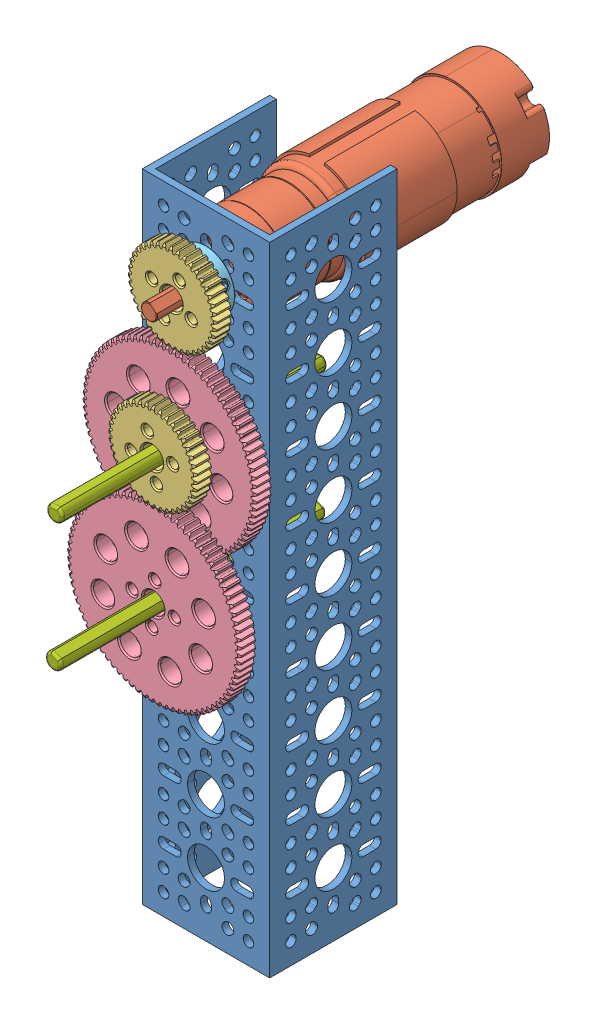
SolidWorks assembly Assem1, configuration Default. Lengths in mm.
Overall size (78.18 240 168.87).
13 component instances, 7 part files, 26 mates.
Components (placement in the parent):
- 1120-0009-0240.step-1: 1120-0009-0240.step [Default] at (-49.2711 21.1308 268.2009) size (48 240 48)
- 5202-0002-0005 part.step-1: 5202-0002-0005 part.step [Default] at (-49.2711 237.1308 159.7009) x (-0.98793 -0.154902 0) z (0 0 -1) size (37.5 37.5 132.7)
- 39028_txm-gear40-tooth.step-1: 39028_txm-gear40-tooth.step [Default] at (-57.5627 238.2461 262.6244) x (0 0 -1) z (0.931474 -0.363809 0) size (6.36 33.59 33.59)
- 39086_txm-gear80-tooth.step-1: 39086_txm-gear80-tooth.step [Default] at (-74.7566 190.6526 244.0115) x (0 0 -1) z (0.976544 0.21532 0) size (6.37 65.59 65.59)
- 39079_txm-motor shaft hub with set screw.step-1: 39079_txm-motor shaft hub with set screw.step [Default] at (-48.4472 172.174 260.2532) x (0.976544 0.21532 0) z (0 0 1) size (22 22 9.4)
- 39079_txm-motor shaft hub with set screw.step-2: 39079_txm-motor shaft hub with set screw.step [Default] at (-58.0114 222.5768 259.2532) x (0.931474 -0.363809 0) z (0 0 1) size (22 22 9.4)
- 1611-0514-0006.step-2: 1611-0514-0006.step [Default] at (-49.2711 189.1308 266.7009) x (0.573511 -0.819198 0) z (-0.819198 -0.573511 0) size (15 5 15)
- 44708_txp-6mm x 100mmaxle.step-1: 44708_txp-6mm x 100mmaxle.step [Default] at (-88.0698 144.3324 212.7991) x (0.997363 0.072577 0) z (0 0 1) size (6 5.5 100)
- 39028_txm-gear40-tooth.step-2: 39028_txm-gear40-tooth.step [Default] at (-56.7838 185.4492 269.9744) x (0 0 -1) z (0.976544 0.21532 0) size (6.36 33.59 33.59)
- 1611-0514-0006.step-3: 1611-0514-0006.step [Default] at (-49.2711 141.1308 266.7009) x (0.943683 0.33085 0) z (0.33085 -0.943683 0) size (15 5 15)
- 44708_txp-6mm x 100mmaxle.step-2: 44708_txp-6mm x 100mmaxle.step [Default] at (-102.7457 115.5828 213.2481) x (0.943185 -0.332267 0) z (0 0 1) size (6 5.5 100)
- 39086_txm-gear80-tooth.step-2: 39086_txm-gear80-tooth.step [Default] at (-73.2644 149.8572 249.8615) x (0 0 -1) z (0.997397 -0.072107 0) size (6.37 65.59 65.59)
- 39079_txm-motor shaft hub with set screw.step-3: 39079_txm-motor shaft hub with set screw.step [Default] at (-53.317 124.6432 266.1032) x (0.997397 -0.072107 0) z (0 0 1) size (22 22 9.4)
Mates (geometry in assembly coordinates):
- Coincident1: coincident: circle of 1120-0009-0240.step-1; circle of 5202-0002-0005 part.step-1
- Concentric2: concentric: circle of 1120-0009-0240.step-1; circle of 5202-0002-0005 part.step-1
- Concentric7: concentric: cylinder of 39086_txm-gear80-tooth.step-1 through (-49.2711 189.1308 231.5757) axis (0 0 1) radius 4; cylinder of 39079_txm-motor shaft hub with set screw.step-1 through (-49.2711 189.1308 281.1009) axis (0 0 -1) radius 3.9625
- Concentric8: concentric: cylinder of 39086_txm-gear80-tooth.step-1 through (-47.5486 181.3184 289.9834) axis (0 0 -1) radius 1.85; circle of 39079_txm-motor shaft hub with set screw.step-1
- Coincident8: coincident: plane of 39086_txm-gear80-tooth.step-1 through (-49.2711 189.1308 278.4009) normal (0 0 -1); plane of 39079_txm-motor shaft hub with set screw.step-1 through (-49.2711 189.1308 278.4009) normal (0 0 1)
- Concentric9: concentric: cylinder of 39028_txm-gear40-tooth.step-1 through (-49.2711 237.1308 230.5758) axis (0 0 1) radius 4; cylinder of 39079_txm-motor shaft hub with set screw.step-2 through (-49.2711 237.1308 280.1009) axis (0 0 -1) radius 3.9625
- Concentric10: concentric: cylinder of 39028_txm-gear40-tooth.step-1 through (-52.1816 229.679 283.7509) axis (0 0 -1) radius 1.85; cylinder of 39079_txm-motor shaft hub with set screw.step-2 through (-52.1816 229.679 270.7009) axis (0 0 1) radius 1.35
- Coincident9: coincident: plane of 39028_txm-gear40-tooth.step-1 through (-49.2711 237.1308 277.4009) normal (0 0 -1); plane of 39079_txm-motor shaft hub with set screw.step-2 through (-49.2711 237.1308 277.4009) normal (0 0 1)
- Concentric11: concentric: cylinder of 5202-0002-0005 part.step-1 through (-49.2711 237.1308 292.2009) axis (0 0 -1) radius 3; cylinder of 39079_txm-motor shaft hub with set screw.step-2 through (-49.2711 237.1308 270.7009) axis (0 0 1) radius 3.015
- Concentric12: concentric: cylinder of 1120-0009-0240.step-1 through (-49.2711 189.1308 260.7009) axis (0 0 1) radius 7; cylinder of 1611-0514-0006.step-2 through (-49.2711 189.1308 270.7009) axis (0 0 -1) radius 7
- Coincident10: coincident: plane of 1120-0009-0240.step-1 through (-25.2711 261.1308 270.7009) normal (0 0 1); plane of 1611-0514-0006.step-2 through (-49.2711 189.1308 270.7009) normal (0 0 -1)
- Concentric13: concentric: cylinder of 1611-0514-0006.step-2 through (-49.2711 189.1308 266.7009) axis (0 0 1) radius 3; cylinder of 44708_txp-6mm x 100mmaxle.step-1 through (-49.2711 189.1308 327.9195) axis (0 0 -1) radius 3
- Concentric14: concentric: cylinder of 39079_txm-motor shaft hub with set screw.step-1 through (-49.2711 189.1308 271.7009) axis (0 0 1) radius 3.015; cylinder of 44708_txp-6mm x 100mmaxle.step-1 through (-49.2711 189.1308 327.9195) axis (0 0 -1) radius 3
- Coincident11: coincident: plane of 39079_txm-motor shaft hub with set screw.step-1 through (-49.2711 189.1308 271.7009) normal (0 0 -1); plane of 1611-0514-0006.step-2 through (-49.2711 189.1308 271.7009) normal (0 0 1)
- Coincident12: coincident: plane of 1120-0009-0240.step-1 through (-25.2711 261.1308 270.7009) normal (0 0 1); plane of 39079_txm-motor shaft hub with set screw.step-2 through (-49.2711 237.1308 270.7009) normal (0 0 -1)
- Concentric15: concentric: cylinder of 44708_txp-6mm x 100mmaxle.step-1 through (-49.2711 189.1308 327.9195) axis (0 0 -1) radius 3; cylinder of 39028_txm-gear40-tooth.step-2 through (-49.2711 189.1308 237.9258) axis (0 0 1) radius 4
- Concentric16: concentric: cylinder of 39086_txm-gear80-tooth.step-1 through (-50.9937 196.9431 289.9834) axis (0 0 -1) radius 1.85; cylinder of 39028_txm-gear40-tooth.step-2 through (-50.9937 196.9431 291.1009) axis (0 0 -1) radius 1.85
- Coincident13: coincident: plane of 39086_txm-gear80-tooth.step-1 through (-49.2711 189.1308 284.7509) normal (0 0 1); plane of 39028_txm-gear40-tooth.step-2 through (-49.2711 189.1308 284.7509) normal (0 0 -1)
- Concentric17: concentric: cylinder of 1120-0009-0240.step-1 through (-49.2711 141.1308 260.7009) axis (0 0 1) radius 7; cylinder of 1611-0514-0006.step-3 through (-49.2711 141.1308 270.7009) axis (0 0 -1) radius 7
- Coincident14: coincident: plane of 1120-0009-0240.step-1 through (-25.2711 261.1308 270.7009) normal (0 0 1); plane of 1611-0514-0006.step-3 through (-49.2711 141.1308 270.7009) normal (0 0 -1)
- Concentric18: concentric: cylinder of 1611-0514-0006.step-3 through (-49.2711 141.1308 266.7009) axis (0 0 1) radius 3; cylinder of 44708_txp-6mm x 100mmaxle.step-2 through (-49.2711 141.1308 328.3684) axis (0 0 -1) radius 3
- Concentric19: concentric: cylinder of 44708_txp-6mm x 100mmaxle.step-2 through (-49.2711 141.1308 328.3684) axis (0 0 -1) radius 3; cylinder of 39086_txm-gear80-tooth.step-2 through (-49.2711 141.1308 237.4257) axis (0 0 1) radius 4
- Coincident15: coincident: circle of 39086_txm-gear80-tooth.step-1; plane of 39086_txm-gear80-tooth.step-2 through (-49.2711 141.1308 284.2509) normal (0 0 -1)
- Concentric20: concentric: cylinder of 44708_txp-6mm x 100mmaxle.step-2 through (-49.2711 141.1308 328.3684) axis (0 0 -1) radius 3; cylinder of 39079_txm-motor shaft hub with set screw.step-3 through (-49.2711 141.1308 277.5509) axis (0 0 1) radius 3.015
- Coincident16: coincident: plane of 39086_txm-gear80-tooth.step-2 through (-49.2711 141.1308 284.2509) normal (0 0 -1); plane of 39079_txm-motor shaft hub with set screw.step-3 through (-49.2711 141.1308 284.2509) normal (0 0 1)
- Concentric21: concentric: cylinder of 39086_txm-gear80-tooth.step-2 through (-48.6943 149.11 295.8334) axis (0 0 -1) radius 1.85; circle of 39079_txm-motor shaft hub with set screw.step-3
